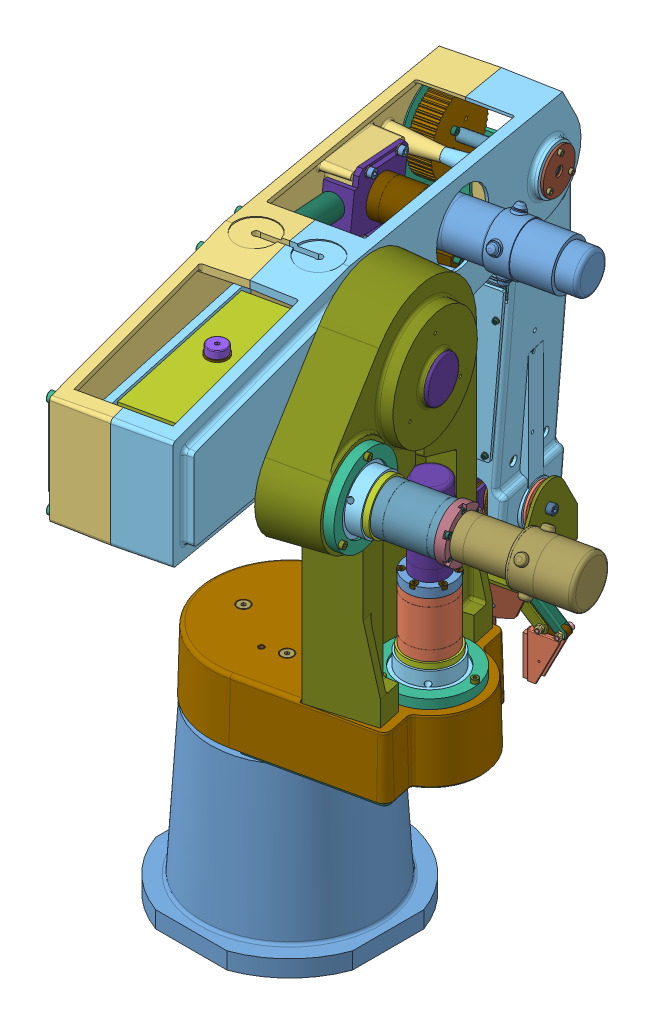
SolidWorks assembly Robot_ericc, configuration Défaut. Lengths in mm. (continued)
Components (placement in the parent): (continued)
- SE-AvtBras-1: SE-AvtBras [Défaut] at (-61.3918 532.5 -273.1877) x (0 1 0) z (-0.977211 0 0.212271) size (419.1 115.2 105.3)
  - AvtBrasD-1: AvtBrasD [Défaut] at origin size (406.26 90.38 52)
  - AvtBrasG-1: AvtBrasG [Défaut] at (-0.1665 0.8325 0) size (406.15 90.36 52)
  - parallel pin hardened_iso-1: parallel pin hardened_iso [Goupille  - 4 x 16 - A - St] at (-265.5 30.1675 -8) x (0 0 1) z (-0.010471 -0.999945 0) size (16 4 4)
  - Vis C HC, M 6x70-1: Vis C HC, M 6x70 [Défaut] at (-65 -16 45.5) x (1 0 0) z (0 -1 0) size (10 76 10)
  - GoupillePosition-1: GoupillePosition [Défaut] at (-65 -16 0.2) x (0 0 1) z (-0.991523 0.129934 0) size (10 8 8)
  - Support moteur-1: Support moteur [Défaut] at (-98.931 38.4675 -40.5) x (0 0 1) z (1 0 0) size (77 78 106) (hidden)
  - socket head cap screw_iso-1: socket head cap screw_iso [Vis CHC M5 x 12 --- 12N] at (-173.5 -4.3325 -27.8) x (0 0 -1) z (0.120643 0.992696 0) size (17 8.5 8.5)
  - socket head cap screw_iso-2: socket head cap screw_iso [Vis CHC M5 x 12 --- 12N] at (-153.5 -4.3325 -27.8) x (0 0 -1) z (0.975756 0.218862 0) size (17 8.5 8.5)
  - plain washer large grade ac_iso-1: plain washer large grade ac_iso [Rondelle M5 Washer ISO 7093 - 5] at (-173.5 -4.3325 -32.8) x (0 0 1) z (-1 0 0) size (1.2 15 15)
  - plain washer large grade ac_iso-3: plain washer large grade ac_iso [Rondelle M5 Washer ISO 7093 - 5] at (-153.5 -4.3325 -32.8) x (0 0 1) z (-1 0 0) size (1.2 15 15)
  - Poulie_M300-006-1: Poulie_M300-006 [Défaut] at (0 0 39) x (0 0 1) z (-0.707107 -0.707107 0) size (22 81.46 81.46)
  - Goupille Cylindrique type A  , 4x24-1: Goupille Cylindrique type A  , 4x24 [Défaut] at (9.1924 9.1924 26.3203) x (0.697271 -0.716808 0) z (0 0 1) size (4 4 24)
  - Goupille Cylindrique type A  , 4x24-3: Goupille Cylindrique type A  , 4x24 [Défaut] at (-9.1924 -9.1924 24.7225) x (-0.993131 -0.117006 0) z (0 0 1) size (4 4 24)
  - socket head cap screw_iso-3: socket head cap screw_iso [Vis CHC M4 x 25 ] at (-9.1924 9.1924 20) x (0 0 1) z (-1 0 0) size (29 7 7)
  - socket head cap screw_iso-4: socket head cap screw_iso [Vis CHC M4 x 25 ] at (9.1924 -9.1924 20) x (0 0 1) z (-1 0 0) size (29 7 7)
  - Came M300 008-1: Came M300 008 [Default] at (0 0 -43) x (0.999885 0.015178 0) z (0 0 1) size (76.42 80 10)
  - parallel pin hardened_iso-2: parallel pin hardened_iso [Goupille  - 4 x 16 - A - St] at (-6.5 -11.2583 -51.3276) x (0 0 1) z (-0.969957 0.243275 0) size (16 4 4)
  - socket head cap screw_iso-5: socket head cap screw_iso [CHC M4 x 16 --- 16N] at (-12.9985 -0.1973 -29) x (0 0 -1) z (-0.999639 0.026878 0) size (20 7 7)
  - socket head cap screw_iso-10: socket head cap screw_iso [CHC M4 x 16 --- 16N] at (6.6701 -11.1584 -29) x (0 0 -1) z (-0.999639 0.026878 0) size (20 7 7)
  - socket head cap screw_iso-12: socket head cap screw_iso [CHC M4 x 16 --- 16N] at (6.3284 11.3557 -29) x (0 0 -1) z (-0.999639 0.026878 0) size (20 7 7)
  - plain washer small grade a_iso-1: plain washer small grade a_iso [Washer M 4] at (-265.5 -21.8325 -8) x (0 0 1) z (-1 0 0) size (0.5 8 8)
  - socket head cap screw_iso-18: socket head cap screw_iso [CHC M4 x 16 --- 16N] at (-265.5 -21.8325 -12.5) x (0 0 1) z (-1 0 0) size (20 7 7)
  - plain washer small grade a_iso-3: plain washer small grade a_iso [Washer M 4] at (-265.5 23.1675 -8) x (0 0 1) z (-1 0 0) size (0.5 8 8)
  - socket head cap screw_iso-19: socket head cap screw_iso [CHC M4 x 16 --- 16N] at (-265.5 23.1675 -12.5) x (0 0 1) z (-1 0 0) size (20 7 7)
  - plain washer small grade a_iso-5: plain washer small grade a_iso [Washer M 4] at (-43.253 27.1675 -8) x (0 0 1) z (-1 0 0) size (0.5 8 8)
  - socket head cap screw_iso-20: socket head cap screw_iso [CHC M4 x 16 --- 16N] at (-43.253 27.1675 -12.5) x (0 0 1) z (-1 0 0) size (20 7 7)
  - moteur poignet-1: moteur poignet [Défaut] at (-218.4709 19.4675 19.5) size (70.8 35 35)
  - socket head cap screw_iso-21: socket head cap screw_iso [ISO 4762 M2 x 6 --- 6N] at (-174.931 8.4675 19.5) x (-1 0 0) z (0 0.924225 0.381849) size (8 3.8 3.8)
  - socket head cap screw_iso-22: socket head cap screw_iso [ISO 4762 M2 x 6 --- 6N] at (-174.931 19.4675 8.5) x (-1 0 0) z (0 -0.381849 0.924225) size (8 3.8 3.8)
  - socket head cap screw_iso-23: socket head cap screw_iso [ISO 4762 M2 x 6 --- 6N] at (-174.931 30.4675 19.5) x (-1 0 0) z (0 -0.924225 -0.381849) size (8 3.8 3.8)
  - socket head cap screw_iso-24: socket head cap screw_iso [ISO 4762 M2 x 6 --- 6N] at (-174.931 19.4675 30.5) x (-1 0 0) z (0 0.381849 -0.924225) size (8 3.8 3.8)
  - Vis CS, M 4x55-1: Vis CS, M 4x55 [Défaut] at (-88.5 -0.5325 -38.5) x (0 -1 0) z (0 0 1) size (7 57.41 7)
  - hex thin nut gradeb_iso-1: hex thin nut gradeb_iso [Hexagon Nut ISO - 4036 - M4 - N] at (-96.731 -0.5325 -38.5) x (0 -0.306361 -0.951915) z (1 0 0) size (7 8.08 2.2)
  - Accouplement flexible-1: Accouplement flexible [Default] at (-161.451 19.4675 19.5) x (-1 0 0) z (0 0.117803 -0.993037) size (17.76 9.53 9.53)
  - Codeur poignet-1: Codeur poignet [Défaut] at (-230.631 -7.9406 32.9669) x (0 0.056728 -0.99839) z (1 0 0) size (30 41.1 18.3)
  - RÇducteur-1: RÇducteur [Défaut] at (-143.931 29.4675 5.5) x (1 0 0) z (0 0 -1) size (82 70 28)
  - radial ball bearing_68_iso-1: radial ball bearing_68_iso [RBB - 1810 - 14,SI,NC,14_68] at (-317.5 -0.8325 -38.5) x (0 0 1) z (-0.812829 -0.582503 0) size (5 19 19)
  - plain washer small grade a_iso-6: plain washer small grade a_iso [Washer courte m5 7092 - 5] at (-138.931 7.4675 33.5) x (0 0 -1) z (1 0 0) size (1 9 9)
  - socket head cap screw_iso-25: socket head cap screw_iso [vis chc M5 x 35 --- 22N] at (-138.931 7.4675 39.5) x (0 0 -1) z (0.75446 0.656346 0) size (40 8.5 8.5)
  - plain washer small grade a_iso-7: plain washer small grade a_iso [Washer courte m5 7092 - 5] at (-88.931 7.4675 33.5) x (0 0 -1) z (1 0 0) size (1 9 9)
  - plain washer small grade a_iso-8: plain washer small grade a_iso [Washer courte m5 7092 - 5] at (-88.931 -35.5325 33.5) x (0 0 -1) z (1 0 0) size (1 9 9)
  - socket head cap screw_iso-26: socket head cap screw_iso [vis chc M5 x 35 --- 22N] at (-88.931 7.4675 39.5) x (0 0 -1) z (0.75446 0.656346 0) size (40 8.5 8.5)
  - socket head cap screw_iso-27: socket head cap screw_iso [vis chc M5 x 35 --- 22N] at (-88.931 -35.5325 39.5) x (0 0 -1) z (0.75446 0.656346 0) size (40 8.5 8.5)
  - Couvercle-3: Couvercle [Défaut] at (-317.5 -0.8325 -49.8) x (-0.559761 -0.828654 0) z (-0.828654 0.559761 0) size (41 8.8 41)
  - socket head cap screw_iso-28: socket head cap screw_iso [Vis CHC M3x8] at (-310.5 11.2918 -52.8) x (0 0 1) z (-0.923728 -0.383049 0) size (11 5.5 5.5)
  - socket head cap screw_iso-29: socket head cap screw_iso [Vis CHC M3x8] at (-310.5 -12.9569 -52.8) x (0 0 1) z (0.130134 0.991496 0) size (11 5.5 5.5)
  - socket head cap screw_iso-30: socket head cap screw_iso [Vis CHC M3x8] at (-331.5 -0.8325 -52.8) x (0 0 1) z (0.793594 -0.608447 0) size (11 5.5 5.5)
  - radial ball bearing_68_iso-4: radial ball bearing_68_iso [RBB - 1810 - 14,SI,NC,14_68] at (-317.5 -0.8325 38.2) x (0 0 1) z (-0.978908 -0.204302 0) size (5 19 19)
  - Couvercle-4: Couvercle [Défaut] at (-317.5 -0.8325 49.5) x (0.997516 0.070441 0) z (-0.070441 0.997516 0) size (41 8.8 41)
  - socket head cap screw_iso-31: socket head cap screw_iso [Vis CHC M3x8] at (-310.5 11.2918 52.5) x (0 0 -1) z (1 0 0) size (11 5.5 5.5)
  - socket head cap screw_iso-32: socket head cap screw_iso [Vis CHC M3x8] at (-331.5 -0.8325 52.5) x (0 0 -1) z (-0.5 0.866025 0) size (11 5.5 5.5)
  - socket head cap screw_iso-33: socket head cap screw_iso [Vis CHC M3x8] at (-310.5 -12.9569 52.5) x (0 0 -1) z (-0.5 -0.866025 0) size (11 5.5 5.5)
  - Capot Superieur_plexi-1: Capot Superieur_plexi [Défaut] at (-81.8928 43.8087 0) x (1 0 0) z (0 1 0) size (220 89.9 3.57)
  - plain washer 10673 type snl_iso-1: plain washer 10673 type snl_iso [rondelle M2] at (-264 46.4087 28) x (0 -1 0) z (0 0 1) size (0.6 6 6)
  - socket head cap screw_iso-34: socket head cap screw_iso [ISO 4762 M2.5 x 10 --- 10N] at (-264 48.9087 28) x (0 -1 0) z (0 0 1) size (12.5 4.5 4.5)
  - plain washer 10673 type snl_iso-9: plain washer 10673 type snl_iso [rondelle M2] at (-264 46.4087 -28) x (0 -1 0) z (0 0 1) size (0.6 6 6)
  - plain washer 10673 type snl_iso-11: plain washer 10673 type snl_iso [rondelle M2] at (-54 46.4087 -40) x (0 -1 0) z (0 0 1) size (0.6 6 6)
  - plain washer 10673 type snl_iso-13: plain washer 10673 type snl_iso [rondelle M2] at (-54 46.4087 40) x (0 -1 0) z (0 0 1) size (0.6 6 6)
  - socket head cap screw_iso-35: socket head cap screw_iso [ISO 4762 M2.5 x 10 --- 10N] at (-264 48.9087 -28) x (0 -1 0) z (0 0 1) size (12.5 4.5 4.5)
  - socket head cap screw_iso-36: socket head cap screw_iso [ISO 4762 M2.5 x 10 --- 10N] at (-54 48.9087 -40) x (0 -1 0) z (0 0 1) size (12.5 4.5 4.5)
  - socket head cap screw_iso-37: socket head cap screw_iso [ISO 4762 M2.5 x 10 --- 10N] at (-54 48.9087 40) x (0 -1 0) z (0 0 1) size (12.5 4.5 4.5)
  - Capot inferieur_plexi-1: Capot inferieur_plexi [Défaut] at (-207.8847 -47.4738 0) x (1 0 0) z (0 1 0) size (165 92.79 3.62)
  - plain washer 10673 type snl_iso-14: plain washer 10673 type snl_iso [rondelle M2] at (-121.3236 -48.0738 -40) x (0 1 0) z (-1 0 0) size (0.6 6 6)
  - plain washer 10673 type snl_iso-16: plain washer 10673 type snl_iso [rondelle M2] at (-121.3236 -48.0738 40) x (0 1 0) z (-1 0 0) size (0.6 6 6)
  - plain washer 10673 type snl_iso-18: plain washer 10673 type snl_iso [rondelle M2] at (-251.3236 -48.0738 30) x (0 1 0) z (-1 0 0) size (0.6 6 6)
  - plain washer 10673 type snl_iso-20: plain washer 10673 type snl_iso [rondelle M2] at (-251.3236 -48.0738 -30) x (0 1 0) z (-1 0 0) size (0.6 6 6)
  - socket head cap screw_iso-38: socket head cap screw_iso [ISO 4762 M2.5 x 10 --- 10N] at (-251.3236 -50.5738 -30) x (0 1 0) z (0 0 1) size (12.5 4.5 4.5)
  - socket head cap screw_iso-39: socket head cap screw_iso [ISO 4762 M2.5 x 10 --- 10N] at (-251.3236 -50.5738 30) x (0 1 0) z (0 0 -1) size (12.5 4.5 4.5)
  - socket head cap screw_iso-40: socket head cap screw_iso [ISO 4762 M2.5 x 10 --- 10N] at (-121.3236 -50.5738 40) x (0 1 0) z (0 0 -1) size (12.5 4.5 4.5)
  - socket head cap screw_iso-41: socket head cap screw_iso [ISO 4762 M2.5 x 10 --- 10N] at (-121.3236 -50.5738 -40) x (0 1 0) z (0 0 -1) size (12.5 4.5 4.5)
  - radial ball bearing_68_skf-1: radial ball bearing_68_skf [Roulement à billes 618-8] at (-113.931 -10.5325 -32.5) x (0 0 -1) z (1 0 0) size (4 16 16)
  - Arbre rÇducteur-1: Arbre rÇducteur [Défaut] at (-113.931 -10.5325 33.5) size (8 8 68)
  - Entretoise-1: Entretoise [Défaut] at (-113.931 -10.5325 -10.5) size (12 12 16)
- Arbre moteur Lacet-1: Arbre moteur Lacet [Défaut] at (122.0871 255.5 -29.1721) x (0 -1 0) z (-0.495579 0 0.868563) size (78.5 36.84 36.92)
  - entraineur-1: entraineur [Défaut] at origin size (78.5 20 20)
  - PoulieE lacet-1: PoulieE lacet [Défaut] at (49 0 0) x (0 -1 0) z (-1 0 0) size (36.84 36.92 30)
  - socket set screw flat point_iso-1: socket set screw flat point_iso [ISO 4026 - M8 x 10-N] at (49 0 16.5) x (0 0 -1) z (1 0 0) size (10 8 8)
  - socket set screw flat point_iso-2: socket set screw flat point_iso [ISO 4026 - M8 x 10-N] at (-7.2554 0 12.9535) x (0 0 -1) z (0.96252 -0.271209 0) size (10 8 8)
- A-M_Epaule-1: A-M_Epaule [Défaut] at (143.3488 474.5 66.3524) x (-0.977211 0 0.212271) z (-0.212271 0 -0.977211) size (78.5 36.84 36.92)
  - entraineur-1: entraineur [Défaut] at origin size (78.5 20 20)
  - P-E_Epaule-1: P-E_Epaule [Défaut] at (49 0 0) x (0 -1 0) z (-1 0 0) size (36.84 36.92 30)
  - socket set screw flat point_iso-1: socket set screw flat point_iso [ISO 4026 - M8 x 10-N] at (49 0 16.5) x (0 0 -1) z (1 0 0) size (10 8 8)
  - socket set screw flat point_iso-2: socket set screw flat point_iso [ISO 4026 - M8 x 10-N] at (-7.2554 0 12.9535) x (0 0 -1) z (0.96252 -0.271209 0) size (10 8 8)
- Poulie_M300-007-1: Poulie_M300-007 [Défaut] at (-55.3873 549.2909 -151.3264) x (0.977211 0 -0.212271) z (0.17106 -0.592111 0.787492) size (27 22.5 22.65)
- Poulie Poignet-1: Poulie Poignet [Défaut] at (-39.1232 418.569 -267.2467) x (-0.212271 0 -0.977211) z (0.977211 0 -0.212271) size (27.43 27.43 20)
- poulie pivotement poignet-1: poulie pivotement poignet [Défaut] at (-76.1895 174.3879 -240.3141) x (-0.99945 0 0.033175) z (0 -1 0) size (20 20 14)
- Support_poignet-1: Support_poignet [Défaut] at (-61.215 215 -272.3741) x (0 1 0) z (-0.977211 0 0.212271) size (98.66 84.05 127)
  - Support-1: Support [Défaut] at origin size (81.5 81.2 115)
  - Assemblage axe pince-1: Assemblage axe pince [Défaut] at (-13.5 0 0) x (0 0 -1) z (1 0 0) size (109 40 59)
    - partie centrale axe avant bras-1: partie centrale axe avant bras [Défaut] at origin size (12 40 21)
    - intÇrieur piäce centrale-1: intÇrieur piäce centrale [Défaut] at (-3 1.5 5) size (6 15.94 13)
    - intÇrieur piäce centrale-2: intÇrieur piäce centrale [Défaut] at (3 -1.5 5) x (-1 0 0) z (0 0 1) size (6 15.94 13)
    - cotÇ axe avant bras-1: cotÇ axe avant bras [Défaut] at (-6 1.807 8.3053) x (1 0 0) z (0 0.944488 0.328546) size (48.5 11 11)
    - cotÇ axe avant bras-2: cotÇ axe avant bras [Défaut] at (6 -1.6292 8.2468) x (-1 0 0) z (0 -0.95512 0.296219) size (48.5 11 11)
    - axe roulements-1: axe roulements [Défaut] x (0 0 -1) z (0.989499 0.144542 0) size (38 10.89 10.89)
  - Assemblage support moteur-1: Assemblage support moteur [Défaut] at (-44.3507 -38.7833 30.5386) x (-1 0 0) z (0 0 -1) size (78.32 60.15 22.52)
    - Support moteur + axe-1: Support moteur + axe [Défaut] at origin size (75.82 60.15 22.2)
    - capteur sur support moteur-1: capteur sur support moteur [Défaut] at (-40.0112 47.5459 15.95) x (0 -0.781659 -0.623706) z (1 0 0) size (6.5 6.5 27.6)
    - plaque avant support moteur-1: plaque avant support moteur [Défaut] at (14.8869 1.1807 -1.9) x (0 0 -1) z (1 0 0) size (22 24 2.5)
  - Ecrou hexagonal ISO 4032, M 9-1: Ecrou hexagonal ISO 4032, M 9 [Défaut] at (-44.23 0 0) x (0 1 0) z (0 0 1) size (16.17 6.98 14)
  - moteur pivotement poignet-1: moteur pivotement poignet [Défaut] at (-26.4843 -28.1507 21.4386) x (-1 0 0) z (0 -0.157023 -0.987595) size (81.2 19.59 19.59)
    - rÇducteur micromoteur-1: rÇducteur micromoteur [Défaut] at origin size (48.3 16 16)
    - micromoteur-1: micromoteur [Défaut] at (-2.1408 0 0) x (1 0 0) z (0 -0.965969 0.258658) size (41 16 16)
  - Poulie axe poignet-1: Poulie axe poignet [Défaut] at (0 0 -18.0612) x (-0.954858 -0.297063 0) z (0 0 -1) size (58.99 58.99 20)
  - Vis C HC, M 6x16-1: Vis C HC, M 6x16 [Défaut] at (0 0 57.5) x (0.243653 -0.969862 0) z (-0.969862 -0.243653 0) size (10 22.04 10)
  - Vis C HC, M 6x16-2: Vis C HC, M 6x16 [Défaut] at (0 0 -57.5) x (1 0 0) z (0 1 0) size (10 22.04 10)
- PortePince-1: PortePince [Défaut] at (-61.215 215 -272.3741) x (0 1 0) z (0.212271 0 0.977211) size (147.79 157.25 45.47)
  - Corps_poignet-1: Corps_poignet [Défaut] at (-113.4 0 -8.5) x (0 -1 0) z (0 0 1) size (87.98 118.07 45.47)
    - Main-1: Main [Défaut] at origin size (87.98 81.17 33)
    - fourreau de poignet-1: fourreau de poignet [Défaut] at (0 76.4 8.5) x (0 1 0) z (0.435216 0 0.900326) size (46.9 34.05 34.05)
    - Roulement type BC 9x17x4-1: Roulement type BC 9x17x4 [Défaut] at (0 94.9 8.5) x (0 -1 0) z (-0.453716 0 0.891146) size (4 17 17)
    - Roulement type BC 9x17x4-2: Roulement type BC 9x17x4 [Défaut] at (0 71.1711 8.5) x (0 -1 0) z (0 0 1) size (4 17 17)
    - Axe-goupille-1: Axe-goupille [Défaut] at (36.5 37 17) size (3.5 3.5 17)
    - Axe-goupille-2: Axe-goupille [Défaut] at (18.5 37 17) size (3.5 3.5 17)
    - Axe-goupille-3: Axe-goupille [Défaut] at (-18.5 37 17) size (3.5 3.5 17)
    - Axe-goupille-4: Axe-goupille [Défaut] at (-36.5 37 17) size (3.5 3.5 17)
    - Axe-goupille-5: Axe-goupille [Défaut] at (-12.5 10 17) size (3.5 3.5 17)
    - Axe-goupille-6: Axe-goupille [Défaut] at (12.5 10 17) size (3.5 3.5 17)
  - bielle 1-1: bielle 1 [Défaut] at (-106.9547 -75.1317 5.4) x (-0.717304 0.69676 0) z (0 0 -1) size (9.87 58.75 10.8)
  - bielle 1-2: bielle 1 [Défaut] at (-106.9547 75.1317 -5.4) x (-0.717304 -0.69676 0) z (0 0 1) size (9.87 58.75 10.8)
  - bielle 2-1: bielle 2 [Défaut] at (-80.8832 -14.1453 5.4) x (0.717304 -0.69676 0) z (0 0 -1) size (12.5 61.5 10.8)
    - bielle 2-1: bielle 2 [Défaut] at origin size (12.5 61.5 10.8)
    - goupille bielle 2-1: goupille bielle 2 [Défaut] at (6.25 18 10.8) x (-0.698934 -0.715186 0) z (0 0 1) size (3.5 3.5 10.8)
  - bielle 2-2: bielle 2 [Défaut] at (-80.8832 14.1453 -5.4) x (0.717304 0.69676 0) z (0 0 1) size (12.5 61.5 10.8)
    - bielle 2-1: bielle 2 [Défaut] at origin size (12.5 61.5 10.8)
    - goupille bielle 2-1: goupille bielle 2 [Défaut] at (6.25 18 10.8) x (-0.698934 -0.715186 0) z (0 0 1) size (3.5 3.5 10.8)
  - Mors-3: Mors [Défaut] at (-210.2541 103.6501 -0.5) x (-1 0 0) z (0 0 -1) size (60 39.8 20)
    - Bielle 3-1: Bielle 3 [Défaut] at (-104.4629 -50.0022 -4.6) size (9.5 27.5 8.2)
    - goupille-1: goupille [Défaut] at (-106.9629 -37.5022 -0.5) x (0 -0.527582 0.849504) z (-1 0 0) size (4 4 14)
    - mors-1: mors [Défaut] at (-49.5801 -64.5882 6.5) size (48 34 14)
    - ecrou_uni_7474-m4x0_7-4_8-5s-1: ecrou_uni_7474-m4x0_7-4_8-5s [Défaut] at (-99.7129 -32.0022 4.9) x (0.66757 0.744547 0) z (0 0 1) size (7 8.09 4.8)
    - ecrou_uni_7474-m4x0_7-4_8-5s-2: ecrou_uni_7474-m4x0_7-4_8-5s [Défaut] at (-99.7129 -50.0022 4.9) x (0.967807 0.251692 0) z (0 0 1) size (7 8.09 4.8)
    - vis chc M4x16-1: vis chc M4x16 [Default] at (-99.7129 -32.0022 -5.9) x (0.255972 0.966684 0) z (0 0 1) size (7 7 20)
    - vis chc M4x16-2: vis chc M4x16 [Default] at (-99.7129 -50.0022 -5.9) x (-0.658187 0.752854 0) z (0 0 1) size (7 7 20)
    - Vis Chc M4-1: Vis Chc M4 [Default] at (-92.9629 -44.5022 -0.5) x (0 0 1) z (-1 0 0) size (7 7 16)
  - Mors-4: Mors [Défaut] at (-210.2541 -103.6501 0.5) x (-1 0 0) z (0 0 1) size (60 39.8 20)
    - Bielle 3-1: Bielle 3 [Défaut] at (-104.4629 -50.0022 -4.6) size (9.5 27.5 8.2)
    - goupille-1: goupille [Défaut] at (-106.9629 -37.5022 -0.5) x (0 -0.527582 0.849504) z (-1 0 0) size (4 4 14)
    - mors-1: mors [Défaut] at (-49.5801 -64.5882 6.5) size (48 34 14)
    - ecrou_uni_7474-m4x0_7-4_8-5s-1: ecrou_uni_7474-m4x0_7-4_8-5s [Défaut] at (-99.7129 -32.0022 4.9) x (0.66757 0.744547 0) z (0 0 1) size (7 8.09 4.8)
    - ecrou_uni_7474-m4x0_7-4_8-5s-2: ecrou_uni_7474-m4x0_7-4_8-5s [Défaut] at (-99.7129 -50.0022 4.9) x (0.967807 0.251692 0) z (0 0 1) size (7 8.09 4.8)
    - vis chc M4x16-1: vis chc M4x16 [Default] at (-99.7129 -32.0022 -5.9) x (0.255972 0.966684 0) z (0 0 1) size (7 7 20)
    - vis chc M4x16-2: vis chc M4x16 [Default] at (-99.7129 -50.0022 -5.9) x (-0.658187 0.752854 0) z (0 0 1) size (7 7 20)
    - Vis Chc M4-1: Vis Chc M4 [Default] at (-92.9629 -44.5022 -0.5) x (0 0 1) z (-1 0 0) size (7 7 16)
Mates (geometry in assembly coordinates):
- Coaxiale1: concentric aligned: cylinder of Ens_Socle-1/Fourreau_200-604-1 through (0 221.7474 0) axis (0 1 0) radius 23.5; cylinder of SE_Chaise-1/SE-Assise-1/SKF_7204-2 through (0 165.3625 0) axis (0 1 0) radius 23.5
- Coïncidente1: coincident anti-aligned: plane of Ens_Socle-1/Fourreau_200-604-1 through (-1.9708 229.5 23.4172) normal (0 -1 0); plane of SE_Chaise-1/SE-Assise-1/SKF_7204-1 through (20.3016 229.5 -4.4099) normal (0 1 0)
- Coaxiale2: concentric anti-aligned: cylinder of SE_Chaise-1/Dossier-1 through (63.5173 532.5 -13.7908) axis (0.977211 0 -0.212271) radius 23.5; cylinder of Bras-1/AXE_Bras-1/7204_Rlt-Billes-2 through (137.9197 532.5 -29.9526) axis (-0.977211 0 0.212271) radius 23.5
- Coïncidente2: coincident anti-aligned: plane of SE_Chaise-1/Dossier-1 through (124.593 532.5 -27.0578) normal (-0.977211 0 0.212271); plane of Bras-1/AXE_Bras-1/7204_Rlt-Billes-2 through (127.5156 548.0575 -13.6033) normal (0.977211 0 -0.212271)
- Coaxiale3: concentric aligned: cylinder of Bras-1/AXE 04 021 M300 011-1 through (-121.9788 532.5 -260.0268) axis (0.977211 0 -0.212271) radius 6; cylinder of SE-AvtBras-1/AvtBrasG-1 through (-112.2067 532.5 -262.1496) axis (0.977211 0 -0.212271) radius 6
- Coïncidente3: coincident aligned: plane of Bras-1/BrasDroit-2 through (-0.5391 505.7717 6.953) normal (-0.977211 0 0.212271); plane of SE-AvtBras-1/AvtBrasD-1 through (-61.3918 532.5 -273.1877) normal (-0.977211 0 0.212271)
- Coaxiale5: concentric aligned: cylinder of SE_Chaise-1/Moto-rÇducteur lacet-1/SKF 6002-1 through (122.0871 209.2625 -29.1721) axis (0 1 0) radius 7.5; cylinder of Arbre moteur Lacet-1/entraineur-1 through (122.0871 277.7027 -29.1721) axis (0 1 0) radius 7.5
- Coïncidente5: coincident anti-aligned: plane of SE_Chaise-1/Moto-rÇducteur lacet-1/SKF 6002-2 through (127.3321 255.5 -23.3989) normal (0 1 0); plane of Arbre moteur Lacet-1/entraineur-1 through (130.7727 255.5 -24.2163) normal (0 -1 0)
- Coaxiale6: concentric aligned: cylinder of SE_Chaise-1/Moteur Epaule-1/SKF 6002-2 through (98.165 474.5 76.1673) axis (0.977211 0 -0.212271) radius 7.5; cylinder of A-M_Epaule-1/entraineur-1 through (165.0455 474.5 61.6395) axis (0.977211 0 -0.212271) radius 7.5
- Coïncidente6: coincident anti-aligned: plane of SE_Chaise-1/Moteur Epaule-1/SKF 6002-1 through (144.9823 473.2287 73.8728) normal (0.977211 0 -0.212271); plane of A-M_Epaule-1/entraineur-1 through (143.3488 484.5 66.3524) normal (-0.977211 0 0.212271)
- Coaxiale7: concentric anti-aligned: cylinder of Bras-1/MotoReduc_Coude-1/Sortie reduc-1 through (-54.8986 549.2909 -151.4325) axis (0.977211 0 -0.212271) radius 5; cylinder of Poulie_M300-007-1 through (-67.3627 549.2909 -148.725) axis (-0.977211 0 0.212271) radius 5
- Coaxiale8: concentric aligned: cylinder of Bras-1/MotoReduc_Coude-1/Sortie reduc-1 through (-71.8779 552.2514 -151.8675) axis (0.17106 -0.592111 0.787492) radius 1.5; cylinder of Poulie_M300-007-1 through (-72.9599 555.9965 -156.8484) axis (0.17106 -0.592111 0.787492) radius 1.5
- Coaxiale9: concentric aligned: cylinder of SE-AvtBras-1/Arbre rÇducteur-1 through (-25.4422 418.569 -270.2185) axis (-0.977211 0 0.212271) radius 4; cylinder of Poulie Poignet-1 through (-29.3511 418.569 -269.3694) axis (-0.977211 0 0.212271) radius 4
- Coïncidente7: coincident anti-aligned: plane of SE-AvtBras-1/Entretoise-1 through (-48.8953 418.569 -265.124) normal (0.977211 0 -0.212271); plane of Poulie Poignet-1 through (-48.8953 418.569 -265.124) normal (-0.977211 0 0.212271)
- Coaxiale10: concentric anti-aligned: cylinder of Support_poignet-1/Assemblage axe pince-1/axe roulements-1 through (-61.215 163.5 -272.3741) axis (0 1 0) radius 4.5; cylinder of PortePince-1/Corps_poignet-1/fourreau de poignet-1 through (-61.215 146.4624 -272.3741) axis (0 -1 0) radius 11
- Coaxiale11: concentric anti-aligned: cylinder of Support_poignet-1/Assemblage axe pince-1/cotÇ axe avant bras-2 through (-26.0354 215 -280.0159) axis (0.977211 0 -0.212271) radius 5; cylinder of SE-AvtBras-1/radial ball bearing_68_iso-1 through (-3.4252 215 -284.9273) axis (-0.977211 0 0.212271) radius 5
- Coïncidente8: coincident aligned: plane of SE-AvtBras-1/AvtBrasD-1 through (-61.3918 532.5 -273.1877) normal (-0.977211 0 0.212271); plane of Support_poignet-1/Support-1 through (-61.215 215 -272.3741) normal (-0.977211 0 0.212271)
- Coïncidente9: coincident anti-aligned: plane of Support_poignet-1/Assemblage axe pince-1/axe roulements-1 through (-61.215 198.5 -272.3741) normal (0 -1 0); plane of PortePince-1/Corps_poignet-1/Roulement type BC 9x17x4-1 through (-56.476 198.5 -271.1285) normal (0 1 0)
- Coaxiale12: concentric aligned: cylinder of poulie pivotement poignet-1 through (-76.1895 162.3879 -240.3141) axis (0 1 0) radius 1.5; cylinder of Support_poignet-1/moteur pivotement poignet-1/rÇducteur micromoteur-1 through (-76.1895 253.1757 -240.3141) axis (0 1 0) radius 1.5
- Coïncidente10: coincident anti-aligned: plane of poulie pivotement poignet-1 through (-76.1895 174.3879 -240.3141) normal (0 1 0); plane of Support_poignet-1/moteur pivotement poignet-1/rÇducteur micromoteur-1 through (-76.3644 174.3879 -243.4208) normal (0 -1 0)
- Parallèle3: parallel anti-aligned: plane of Ens_Socle-1/Socle-1 through (-113 0 0) normal (0 -1 0); plane of Bras-1/BrasDroit-2
- Parallèle2: parallel aligned: plane of SE-AvtBras-1/AvtBrasD-1; plane of Support_poignet-1/Support-1
- Perpendiculaire1: perpendicular: plane of Ens_Socle-1/Socle-1 through (-113 0 0) normal (0 -1 0); plane of SE-AvtBras-1/AvtBrasD-1
- Coïncidente16: coincident anti-aligned: plane of Support_poignet-1/Support-1; plane of PortePince-1 through (-61.215 215 -272.3741) normal (0.212271 0 0.977211)
